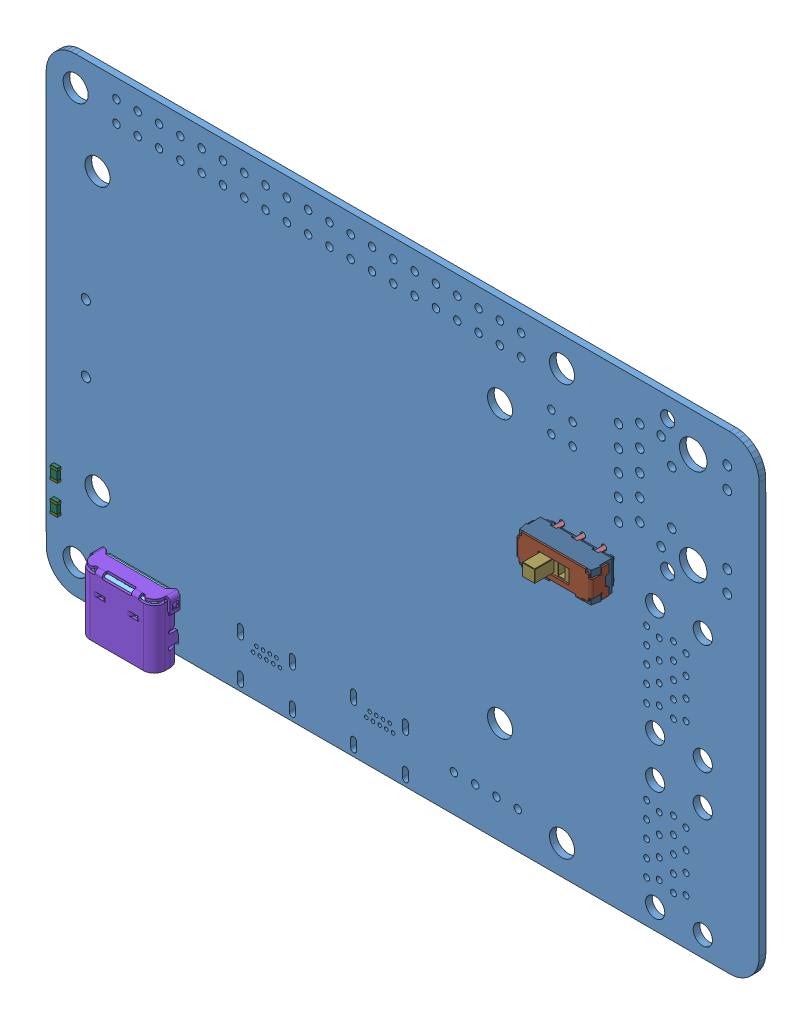
SolidWorks assembly CM4-to-Pi4-Adapter, configuration Default. Lengths in mm.
Overall size (85.02 56.9 9.11).
557 component instances, 55 part files, 0 mates.
Components (placement in the parent):
- CM4-to-Pi4-Adapter-3D.step-1: CM4-to-Pi4-Adapter-3D.step [Default] at origin size (85.02 56.9 9.11)
  - C56.step-1: C56.step [Default] at origin size (1.65 0.7 0.46)
    - 1028708016.step-1: 1028708016.step [Default] at (21.6693 15.4568 -1.2584) size (0.28 0.7 0.46)
      - Extruded.step-1: Extruded.step [Default] at origin size (0.28 0.7 0.46)
    - 1028708016.step-2: 1028708016.step [Default] at (20.2978 15.4568 -1.2584) size (0.28 0.7 0.46)
      - Extruded.step-1: Extruded.step [Default] at origin size (0.28 0.7 0.46)
    - 1028712752.step-1: 1028712752.step [Default] at (20.9835 15.4568 -1.2484) size (1.5 0.6 0.42)
      - Extruded-0.step-1: Extruded-0.step [Default] at origin size (1.5 0.6 0.42)
  - RJ1.step-1: RJ1.step [Default] at origin (suppressed, hidden)
  - C43.step-1: C43.step [Default] at origin size (1.65 0.7 0.46)
    - 1028708016.step-1: 1028708016.step [Default] at (79.781 44.229 -1.2584) size (0.28 0.7 0.46)
      - Extruded.step-1: Extruded.step [Default] at origin size (0.28 0.7 0.46)
    - 1028708016.step-2: 1028708016.step [Default] at (81.1525 44.229 -1.2584) size (0.28 0.7 0.46)
      - Extruded.step-1: Extruded.step [Default] at origin size (0.28 0.7 0.46)
    - 1028712752.step-1: 1028712752.step [Default] at (80.4667 44.229 -1.2484) size (1.5 0.6 0.42)
      - Extruded-0.step-1: Extruded-0.step [Default] at origin size (1.5 0.6 0.42)
  - U5.step-1: U5.step [Default] at origin size (7.8 5.3 2.16)
    - 1028708272.step-1: 1028708272.step [Default] at (47.5222 47.1882 -1.0524) size (1.3 0.41 0.25)
      - Extruded-6.step-1: Extruded-6.step [Default] at origin size (1.3 0.41 0.25)
    - 1028708272.step-2: 1028708272.step [Default] at (47.5222 45.9182 -1.0524) size (1.3 0.41 0.25)
      - Extruded-6.step-1: Extruded-6.step [Default] at origin size (1.3 0.41 0.25)
    - 1028708272.step-3: 1028708272.step [Default] at (47.5222 44.6482 -1.0524) size (1.3 0.41 0.25)
      - Extruded-6.step-1: Extruded-6.step [Default] at origin size (1.3 0.41 0.25)
    - 1028708272.step-4: 1028708272.step [Default] at (47.5222 43.3782 -1.0524) size (1.3 0.41 0.25)
      - Extruded-6.step-1: Extruded-6.step [Default] at origin size (1.3 0.41 0.25)
    - 1028708272.step-5: 1028708272.step [Default] at (41.0222 47.1982 -1.0524) size (1.3 0.41 0.25)
      - Extruded-6.step-1: Extruded-6.step [Default] at origin size (1.3 0.41 0.25)
    - 1028708272.step-6: 1028708272.step [Default] at (41.0222 45.9282 -1.0524) size (1.3 0.41 0.25)
      - Extruded-6.step-1: Extruded-6.step [Default] at origin size (1.3 0.41 0.25)
    - 1028708272.step-7: 1028708272.step [Default] at (41.0222 44.6582 -1.0524) size (1.3 0.41 0.25)
      - Extruded-6.step-1: Extruded-6.step [Default] at origin size (1.3 0.41 0.25)
    - 1028708272.step-8: 1028708272.step [Default] at (41.0222 43.3882 -1.0524) size (1.3 0.41 0.25)
      - Extruded-6.step-1: Extruded-6.step [Default] at origin size (1.3 0.41 0.25)
    - 1028710064.step-1: 1028710064.step [Default] at (44.2722 45.2882 -2.9584) size (5.4 5.3 2.01)
      - Extruded-7.step-1: Extruded-7.step [Default] at origin size (5.4 5.3 2.01)
  - Type_C1.step-1: Type_C1.step [Default] at origin size (9.58 7.71 4.16)
    - 698b116-264-211.step-1: 698b116-264-211.step [Default] at (-4.8722 -5.2197 -12) x (1 0 0) z (0 -1 0) size (9.58 4.16 7.71)
      - SOLID.step-1: SOLID.step [Default] at origin size (8.34 3.56 7.05)
      - SOLID-8.step-1: SOLID-8.step [Default] at origin size (0.26 1.45 0.87)
      - SOLID-9.step-1: SOLID-9.step [Default] at origin size (0.26 1.45 0.87)
      - SOLID-10.step-1: SOLID-10.step [Default] at origin size (0.25 1.45 0.87)
      - SOLID-11.step-1: SOLID-11.step [Default] at origin size (0.25 1.45 0.87)
      - SOLID-12.step-1: SOLID-12.step [Default] at origin size (0.25 2.03 6.58)
      - SOLID-13.step-1: SOLID-13.step [Default] at origin size (0.25 2.03 6.58)
      - SOLID-14.step-1: SOLID-14.step [Default] at origin size (0.25 1.57 6.58)
      - SOLID-15.step-1: SOLID-15.step [Default] at origin size (0.25 1.57 6.58)
      - SOLID-16.step-1: SOLID-16.step [Default] at origin size (0.25 0.24 5.71)
      - SOLID-17.step-1: SOLID-17.step [Default] at origin size (0.25 0.24 5.71)
      - SOLID-18.step-1: SOLID-18.step [Default] at origin size (0.85 1.57 7.13)
      - SOLID-19.step-1: SOLID-19.step [Default] at origin size (0.35 2.03 6.78)
      - SOLID-20.step-1: SOLID-20.step [Default] at origin size (0.35 0.24 5.91)
      - SOLID-21.step-1: SOLID-21.step [Default] at origin size (0.35 2.03 6.78)
      - SOLID-22.step-1: SOLID-22.step [Default] at origin size (0.35 0.24 5.91)
      - SOLID-23.step-1: SOLID-23.step [Default] at origin size (0.85 1.57 7.13)
      - SOLID-24.step-1: SOLID-24.step [Default] at origin size (0.25 0.24 4.21)
      - SOLID-25.step-1: SOLID-25.step [Default] at origin size (0.25 0.24 4.21)
      - SOLID-26.step-1: SOLID-26.step [Default] at origin size (1.11 2.03 7.13)
      - SOLID-27.step-1: SOLID-27.step [Default] at origin size (1.12 2.03 7.13)
      - SOLID-28.step-1: SOLID-28.step [Default] at origin size (9.58 4.16 7.53)
  - PWR4.step-1: PWR4.step [Default] at origin size (1.65 0.7 0.46)
    - 1028708016.step-1: 1028708016.step [Default] at (60.1471 9.525 -1.2584) size (0.28 0.7 0.46)
      - Extruded.step-1: Extruded.step [Default] at origin size (0.28 0.7 0.46)
    - 1028708016.step-2: 1028708016.step [Default] at (61.5187 9.525 -1.2584) size (0.28 0.7 0.46)
      - Extruded.step-1: Extruded.step [Default] at origin size (0.28 0.7 0.46)
    - 1028712752.step-1: 1028712752.step [Default] at (60.8329 9.525 -1.2484) size (1.5 0.6 0.42)
      - Extruded-0.step-1: Extruded-0.step [Default] at origin size (1.5 0.6 0.42)
  - J2.step-1: J2.step [Default] at origin (suppressed, hidden)
  - J1.step-1: J1.step [Default] at origin (suppressed, hidden)
  - I1.step-1: I1.step [Default] at origin size (1.2 2.3 1.1)
    - User_Library-1N4148WS.step-1: User_Library-1N4148WS.step [Default] at (45.6439 39.5224 -1.05) x (0 -1 0) z (0 0 1) size (2.3 1.2 1.1)
  - U6.step-1: U6.step [Default] at origin size (8.1 8.1 0.83)
    - 1028701360.step-1: 1028701360.step [Default] at (46.9011 27.4447 -1.6484) size (8.1 8.1 0.83)
      - Extruded-53.step-1: Extruded-53.step [Default] at origin size (8.1 8.1 0.83)
  - PWR3.step-1: PWR3.step [Default] at origin size (1.65 0.85 0.46)
    - 1032565968.step-1: 1032565968.step [Default] at (60.7531 10.7826 -1.2484) size (1.5 0.8 0.42)
      - Extruded-54.step-1: Extruded-54.step [Default] at origin size (1.5 0.8 0.42)
    - 1032565712.step-1: 1032565712.step [Default] at (60.0673 10.7826 -1.2584) size (0.28 0.85 0.46)
      - Extruded-55.step-1: Extruded-55.step [Default] at origin size (0.28 0.85 0.46)
    - 1032565712.step-2: 1032565712.step [Default] at (61.4388 10.7826 -1.2584) size (0.28 0.85 0.46)
      - Extruded-55.step-1: Extruded-55.step [Default] at origin size (0.28 0.85 0.46)
  - PWR2.step-1: PWR2.step [Default] at origin size (0.7 1.65 0.46)
    - 1028703920.step-1: 1028703920.step [Default] at (53.2384 19.7867 -1.2584) size (0.7 0.28 0.46)
      - Extruded-56.step-1: Extruded-56.step [Default] at origin size (0.7 0.28 0.46)
    - 1028703920.step-2: 1028703920.step [Default] at (53.2384 18.4151 -1.2584) size (0.7 0.28 0.46)
      - Extruded-56.step-1: Extruded-56.step [Default] at origin size (0.7 0.28 0.46)
    - 1032570704.step-1: 1032570704.step [Default] at (53.2384 19.1009 -1.2484) size (0.6 1.5 0.42)
      - Extruded-57.step-1: Extruded-57.step [Default] at origin size (0.6 1.5 0.42)
  - PWR1.step-1: PWR1.step [Default] at origin size (0.85 1.65 0.46)
    - 1032565072.step-1: 1032565072.step [Default] at (54.5845 19.0753 -1.2484) size (0.8 1.5 0.42)
      - Extruded-58.step-1: Extruded-58.step [Default] at origin size (0.8 1.5 0.42)
    - 1032568144.step-1: 1032568144.step [Default] at (54.5845 19.7611 -1.2584) size (0.85 0.28 0.46)
      - Extruded-59.step-1: Extruded-59.step [Default] at origin size (0.85 0.28 0.46)
    - 1032568144.step-2: 1032568144.step [Default] at (54.5845 18.3896 -1.2584) size (0.85 0.28 0.46)
      - Extruded-59.step-1: Extruded-59.step [Default] at origin size (0.85 0.28 0.46)
  - C55.step-1: C55.step [Default] at origin size (0.85 1.65 0.46)
    - 1032568144.step-1: 1032568144.step [Default] at (8.4022 6.793 -1.2584) size (0.85 0.28 0.46)
      - Extruded-59.step-1: Extruded-59.step [Default] at origin size (0.85 0.28 0.46)
    - 1032568144.step-2: 1032568144.step [Default] at (8.4022 8.1646 -1.2584) size (0.85 0.28 0.46)
      - Extruded-59.step-1: Extruded-59.step [Default] at origin size (0.85 0.28 0.46)
    - 1032565072.step-1: 1032565072.step [Default] at (8.4022 7.4787 -1.2484) size (0.8 1.5 0.42)
      - Extruded-58.step-1: Extruded-58.step [Default] at origin size (0.8 1.5 0.42)
  - C54.step-1: C54.step [Default] at origin size (0.85 1.65 0.46)
    - 1032568144.step-1: 1032568144.step [Default] at (39.5479 19.754 -1.2584) size (0.85 0.28 0.46)
      - Extruded-59.step-1: Extruded-59.step [Default] at origin size (0.85 0.28 0.46)
    - 1032568144.step-2: 1032568144.step [Default] at (39.5479 18.3825 -1.2584) size (0.85 0.28 0.46)
      - Extruded-59.step-1: Extruded-59.step [Default] at origin size (0.85 0.28 0.46)
    - 1032565072.step-1: 1032565072.step [Default] at (39.5479 19.0683 -1.2484) size (0.8 1.5 0.42)
      - Extruded-58.step-1: Extruded-58.step [Default] at origin size (0.8 1.5 0.42)
  - C53.step-1: C53.step [Default] at origin size (1.65 0.85 0.46)
    - 1032565712.step-1: 1032565712.step [Default] at (47.5691 18.4938 -1.2584) size (0.28 0.85 0.46)
      - Extruded-55.step-1: Extruded-55.step [Default] at origin size (0.28 0.85 0.46)
    - 1032565712.step-2: 1032565712.step [Default] at (46.1976 18.4938 -1.2584) size (0.28 0.85 0.46)
      - Extruded-55.step-1: Extruded-55.step [Default] at origin size (0.28 0.85 0.46)
    - 1032565968.step-1: 1032565968.step [Default] at (46.8834 18.4938 -1.2484) size (1.5 0.8 0.42)
      - Extruded-54.step-1: Extruded-54.step [Default] at origin size (1.5 0.8 0.42)
  - C52.step-1: C52.step [Default] at origin size (1.65 0.7 0.46)
    - 1028708016.step-1: 1028708016.step [Default] at (53.2841 32.3371 -1.2584) size (0.28 0.7 0.46)
      - Extruded.step-1: Extruded.step [Default] at origin size (0.28 0.7 0.46)
    - 1028708016.step-2: 1028708016.step [Default] at (54.6556 32.3371 -1.2584) size (0.28 0.7 0.46)
      - Extruded.step-1: Extruded.step [Default] at origin size (0.28 0.7 0.46)
    - 1028712752.step-1: 1028712752.step [Default] at (53.9699 32.3371 -1.2484) size (1.5 0.6 0.42)
      - Extruded-0.step-1: Extruded-0.step [Default] at origin size (1.5 0.6 0.42)
  - C51.step-1: C51.step [Default] at origin size (0.7 1.65 0.46)
    - 1028703920.step-1: 1028703920.step [Default] at (44.5186 19.746 -1.2584) size (0.7 0.28 0.46)
      - Extruded-56.step-1: Extruded-56.step [Default] at origin size (0.7 0.28 0.46)
    - 1028703920.step-2: 1028703920.step [Default] at (44.5186 18.3745 -1.2584) size (0.7 0.28 0.46)
      - Extruded-56.step-1: Extruded-56.step [Default] at origin size (0.7 0.28 0.46)
    - 1032570704.step-1: 1032570704.step [Default] at (44.5186 19.0602 -1.2484) size (0.6 1.5 0.42)
      - Extruded-57.step-1: Extruded-57.step [Default] at origin size (0.6 1.5 0.42)
  - C50.step-1: C50.step [Default] at origin size (0.7 1.65 0.46)
    - 1028703920.step-1: 1028703920.step [Default] at (42.1519 19.746 -1.2584) size (0.7 0.28 0.46)
      - Extruded-56.step-1: Extruded-56.step [Default] at origin size (0.7 0.28 0.46)
    - 1028703920.step-2: 1028703920.step [Default] at (42.1519 18.3745 -1.2584) size (0.7 0.28 0.46)
      - Extruded-56.step-1: Extruded-56.step [Default] at origin size (0.7 0.28 0.46)
    - 1032570704.step-1: 1032570704.step [Default] at (42.1519 19.0602 -1.2484) size (0.6 1.5 0.42)
      - Extruded-57.step-1: Extruded-57.step [Default] at origin size (0.6 1.5 0.42)
  - C49.step-1: C49.step [Default] at origin size (0.7 1.65 0.46)
    - 1028703920.step-1: 1028703920.step [Default] at (43.3352 19.746 -1.2584) size (0.7 0.28 0.46)
      - Extruded-56.step-1: Extruded-56.step [Default] at origin size (0.7 0.28 0.46)
    - 1028703920.step-2: 1028703920.step [Default] at (43.3352 18.3745 -1.2584) size (0.7 0.28 0.46)
      - Extruded-56.step-1: Extruded-56.step [Default] at origin size (0.7 0.28 0.46)
    - 1032570704.step-1: 1032570704.step [Default] at (43.3352 19.0602 -1.2484) size (0.6 1.5 0.42)
      - Extruded-57.step-1: Extruded-57.step [Default] at origin size (0.6 1.5 0.42)
  - C48.step-1: C48.step [Default] at origin size (0.7 1.65 0.46)
    - 1028703920.step-1: 1028703920.step [Default] at (49.2404 19.746 -1.2584) size (0.7 0.28 0.46)
      - Extruded-56.step-1: Extruded-56.step [Default] at origin size (0.7 0.28 0.46)
    - 1028703920.step-2: 1028703920.step [Default] at (49.2404 18.3745 -1.2584) size (0.7 0.28 0.46)
      - Extruded-56.step-1: Extruded-56.step [Default] at origin size (0.7 0.28 0.46)
    - 1032570704.step-1: 1032570704.step [Default] at (49.2404 19.0602 -1.2484) size (0.6 1.5 0.42)
      - Extruded-57.step-1: Extruded-57.step [Default] at origin size (0.6 1.5 0.42)
  - C47.step-1: C47.step [Default] at origin size (0.7 1.65 0.46)
    - 1028703920.step-1: 1028703920.step [Default] at (43.3429 34.5262 -1.2584) size (0.7 0.28 0.46)
      - Extruded-56.step-1: Extruded-56.step [Default] at origin size (0.7 0.28 0.46)
    - 1028703920.step-2: 1028703920.step [Default] at (43.3429 35.8977 -1.2584) size (0.7 0.28 0.46)
      - Extruded-56.step-1: Extruded-56.step [Default] at origin size (0.7 0.28 0.46)
    - 1032570704.step-1: 1032570704.step [Default] at (43.3429 35.212 -1.2484) size (0.6 1.5 0.42)
      - Extruded-57.step-1: Extruded-57.step [Default] at origin size (0.6 1.5 0.42)
  - C46.step-1: C46.step [Default] at origin size (1.65 0.7 0.46)
    - 1028708016.step-1: 1028708016.step [Default] at (47.5692 19.812 -1.2584) size (0.28 0.7 0.46)
      - Extruded.step-1: Extruded.step [Default] at origin size (0.28 0.7 0.46)
    - 1028708016.step-2: 1028708016.step [Default] at (46.1976 19.812 -1.2584) size (0.28 0.7 0.46)
      - Extruded.step-1: Extruded.step [Default] at origin size (0.28 0.7 0.46)
    - 1028712752.step-1: 1028712752.step [Default] at (46.8834 19.812 -1.2484) size (1.5 0.6 0.42)
      - Extruded-0.step-1: Extruded-0.step [Default] at origin size (1.5 0.6 0.42)
  - C45.step-1: C45.step [Default] at origin size (1.65 0.7 0.46)
    - 1028708016.step-1: 1028708016.step [Default] at (38.7807 25.7962 -1.2584) size (0.28 0.7 0.46)
      - Extruded.step-1: Extruded.step [Default] at origin size (0.28 0.7 0.46)
    - 1028708016.step-2: 1028708016.step [Default] at (40.1522 25.7962 -1.2584) size (0.28 0.7 0.46)
      - Extruded.step-1: Extruded.step [Default] at origin size (0.28 0.7 0.46)
    - 1028712752.step-1: 1028712752.step [Default] at (39.4664 25.7962 -1.2484) size (1.5 0.6 0.42)
      - Extruded-0.step-1: Extruded-0.step [Default] at origin size (1.5 0.6 0.42)
  - C44.step-1: C44.step [Default] at origin size (1.65 0.7 0.46)
    - 1028708016.step-1: 1028708016.step [Default] at (38.7858 26.8605 -1.2584) size (0.28 0.7 0.46)
      - Extruded.step-1: Extruded.step [Default] at origin size (0.28 0.7 0.46)
    - 1028708016.step-2: 1028708016.step [Default] at (40.1573 26.8605 -1.2584) size (0.28 0.7 0.46)
      - Extruded.step-1: Extruded.step [Default] at origin size (0.28 0.7 0.46)
    - 1028712752.step-1: 1028712752.step [Default] at (39.4715 26.8605 -1.2484) size (1.5 0.6 0.42)
      - Extruded-0.step-1: Extruded-0.step [Default] at origin size (1.5 0.6 0.42)
  - C42.step-1: C42.step [Default] at origin size (1.65 0.7 0.46)
    - 1028708016.step-1: 1028708016.step [Default] at (38.7263 28.1998 -1.2584) size (0.28 0.7 0.46)
      - Extruded.step-1: Extruded.step [Default] at origin size (0.28 0.7 0.46)
    - 1028708016.step-2: 1028708016.step [Default] at (40.0979 28.1998 -1.2584) size (0.28 0.7 0.46)
      - Extruded.step-1: Extruded.step [Default] at origin size (0.28 0.7 0.46)
    - 1028712752.step-1: 1028712752.step [Default] at (39.4121 28.1998 -1.2484) size (1.5 0.6 0.42)
      - Extruded-0.step-1: Extruded-0.step [Default] at origin size (1.5 0.6 0.42)
  - C41.step-1: C41.step [Default] at origin size (1.65 0.7 0.46)
    - 1028708016.step-1: 1028708016.step [Default] at (38.7349 29.243 -1.2584) size (0.28 0.7 0.46)
      - Extruded.step-1: Extruded.step [Default] at origin size (0.28 0.7 0.46)
    - 1028708016.step-2: 1028708016.step [Default] at (40.1065 29.243 -1.2584) size (0.28 0.7 0.46)
      - Extruded.step-1: Extruded.step [Default] at origin size (0.28 0.7 0.46)
    - 1028712752.step-1: 1028712752.step [Default] at (39.4207 29.243 -1.2484) size (1.5 0.6 0.42)
      - Extruded-0.step-1: Extruded-0.step [Default] at origin size (1.5 0.6 0.42)
  - C40.step-1: C40.step [Default] at origin size (0.85 1.65 0.46)
    - 1032565072.step-1: 1032565072.step [Default] at (51.1555 35.2043 -1.2484) size (0.8 1.5 0.42)
      - Extruded-58.step-1: Extruded-58.step [Default] at origin size (0.8 1.5 0.42)
    - 1032568144.step-1: 1032568144.step [Default] at (51.1555 35.8901 -1.2584) size (0.85 0.28 0.46)
      - Extruded-59.step-1: Extruded-59.step [Default] at origin size (0.85 0.28 0.46)
    - 1032568144.step-2: 1032568144.step [Default] at (51.1555 34.5186 -1.2584) size (0.85 0.28 0.46)
      - Extruded-59.step-1: Extruded-59.step [Default] at origin size (0.85 0.28 0.46)
  - C39.step-1: C39.step [Default] at origin size (1.65 0.7 0.46)
    - 1028708016.step-1: 1028708016.step [Default] at (40.1626 31.1912 -1.2584) size (0.28 0.7 0.46)
      - Extruded.step-1: Extruded.step [Default] at origin size (0.28 0.7 0.46)
    - 1028708016.step-2: 1028708016.step [Default] at (38.791 31.1912 -1.2584) size (0.28 0.7 0.46)
      - Extruded.step-1: Extruded.step [Default] at origin size (0.28 0.7 0.46)
    - 1028712752.step-1: 1028712752.step [Default] at (39.4767 31.1912 -1.2484) size (1.5 0.6 0.42)
      - Extruded-0.step-1: Extruded-0.step [Default] at origin size (1.5 0.6 0.42)
  - C38.step-1: C38.step [Default] at origin size (1.65 0.7 0.46)
    - 1028708016.step-1: 1028708016.step [Default] at (40.2336 23.3096 -1.2584) size (0.28 0.7 0.46)
      - Extruded.step-1: Extruded.step [Default] at origin size (0.28 0.7 0.46)
    - 1028708016.step-2: 1028708016.step [Default] at (38.8621 23.3096 -1.2584) size (0.28 0.7 0.46)
      - Extruded.step-1: Extruded.step [Default] at origin size (0.28 0.7 0.46)
    - 1028712752.step-1: 1028712752.step [Default] at (39.5478 23.3096 -1.2484) size (1.5 0.6 0.42)
      - Extruded-0.step-1: Extruded-0.step [Default] at origin size (1.5 0.6 0.42)
  - C37.step-1: C37.step [Default] at origin size (0.7 1.65 0.46)
    - 1028703920.step-1: 1028703920.step [Default] at (50.5973 19.746 -1.2584) size (0.7 0.28 0.46)
      - Extruded-56.step-1: Extruded-56.step [Default] at origin size (0.7 0.28 0.46)
    - 1028703920.step-2: 1028703920.step [Default] at (50.5973 18.3745 -1.2584) size (0.7 0.28 0.46)
      - Extruded-56.step-1: Extruded-56.step [Default] at origin size (0.7 0.28 0.46)
    - 1032570704.step-1: 1032570704.step [Default] at (50.5973 19.0602 -1.2484) size (0.6 1.5 0.42)
      - Extruded-57.step-1: Extruded-57.step [Default] at origin size (0.6 1.5 0.42)
  - C36.step-1: C36.step [Default] at origin size (0.7 1.65 0.46)
    - 1028703920.step-1: 1028703920.step [Default] at (51.9542 19.746 -1.2584) size (0.7 0.28 0.46)
      - Extruded-56.step-1: Extruded-56.step [Default] at origin size (0.7 0.28 0.46)
    - 1028703920.step-2: 1028703920.step [Default] at (51.9542 18.3745 -1.2584) size (0.7 0.28 0.46)
      - Extruded-56.step-1: Extruded-56.step [Default] at origin size (0.7 0.28 0.46)
    - 1032570704.step-1: 1032570704.step [Default] at (51.9542 19.0602 -1.2484) size (0.6 1.5 0.42)
      - Extruded-57.step-1: Extruded-57.step [Default] at origin size (0.6 1.5 0.42)
  - C35.step-1: C35.step [Default] at origin size (1.65 0.7 0.46)
    - 1028708016.step-1: 1028708016.step [Default] at (53.2892 33.4826 -1.2584) size (0.28 0.7 0.46)
      - Extruded.step-1: Extruded.step [Default] at origin size (0.28 0.7 0.46)
    - 1028708016.step-2: 1028708016.step [Default] at (54.6608 33.4826 -1.2584) size (0.28 0.7 0.46)
      - Extruded.step-1: Extruded.step [Default] at origin size (0.28 0.7 0.46)
    - 1028712752.step-1: 1028712752.step [Default] at (53.975 33.4826 -1.2484) size (1.5 0.6 0.42)
      - Extruded-0.step-1: Extruded-0.step [Default] at origin size (1.5 0.6 0.42)
  - C34.step-1: C34.step [Default] at origin size (1.65 0.7 0.46)
    - 1028708016.step-1: 1028708016.step [Default] at (53.2841 22.2834 -1.2584) size (0.28 0.7 0.46)
      - Extruded.step-1: Extruded.step [Default] at origin size (0.28 0.7 0.46)
    - 1028708016.step-2: 1028708016.step [Default] at (54.6556 22.2834 -1.2584) size (0.28 0.7 0.46)
      - Extruded.step-1: Extruded.step [Default] at origin size (0.28 0.7 0.46)
    - 1028712752.step-1: 1028712752.step [Default] at (53.9699 22.2834 -1.2484) size (1.5 0.6 0.42)
      - Extruded-0.step-1: Extruded-0.step [Default] at origin size (1.5 0.6 0.42)
  - C33.step-1: C33.step [Default] at origin size (1.65 0.7 0.46)
    - 1028708016.step-1: 1028708016.step [Default] at (53.2581 21.1786 -1.2584) size (0.28 0.7 0.46)
      - Extruded.step-1: Extruded.step [Default] at origin size (0.28 0.7 0.46)
    - 1028708016.step-2: 1028708016.step [Default] at (54.6296 21.1786 -1.2584) size (0.28 0.7 0.46)
      - Extruded.step-1: Extruded.step [Default] at origin size (0.28 0.7 0.46)
    - 1028712752.step-1: 1028712752.step [Default] at (53.9439 21.1786 -1.2484) size (1.5 0.6 0.42)
      - Extruded-0.step-1: Extruded-0.step [Default] at origin size (1.5 0.6 0.42)
  - AMS-1.step-1: AMS-1.step [Default] at origin size (6.73 3.43 1.02)
    - 1032565584.step-1: 1032565584.step [Default] at (60.7466 16.1548 -2.0684) size (6.73 3.43 1.02)
      - Extruded-60.step-1: Extruded-60.step [Default] at origin size (6.73 3.43 1.02)
  - C9.step-1: C9.step [Default] at origin size (0.7 1.65 0.46)
    - 1028703920.step-1: 1028703920.step [Default] at (38.585 45.8952 -1.2584) size (0.7 0.28 0.46)
      - Extruded-56.step-1: Extruded-56.step [Default] at origin size (0.7 0.28 0.46)
    - 1028703920.step-2: 1028703920.step [Default] at (38.585 47.2668 -1.2584) size (0.7 0.28 0.46)
      - Extruded-56.step-1: Extruded-56.step [Default] at origin size (0.7 0.28 0.46)
    - 1032570704.step-1: 1032570704.step [Default] at (38.585 46.581 -1.2484) size (0.6 1.5 0.42)
      - Extruded-57.step-1: Extruded-57.step [Default] at origin size (0.6 1.5 0.42)
  - C23.step-1: C23.step [Default] at origin size (1.6 0.8 0.6)
    - CAPC1608(0603).step-1: CAPC1608(0603).step [Default] at (20.9711 17.8537 -0.7984) x (-1 0 0) z (0 0 -1) size (1.6 0.8 0.6)
  - P3.step-1: P3.step [Default] at origin (suppressed, hidden)
  - C32.step-1: C32.step [Default] at origin size (0.7 1.65 0.46)
    - 1028703920.step-1: 1028703920.step [Default] at (47.0662 38.9381 -1.2584) size (0.7 0.28 0.46)
      - Extruded-56.step-1: Extruded-56.step [Default] at origin size (0.7 0.28 0.46)
    - 1028703920.step-2: 1028703920.step [Default] at (47.0662 40.3097 -1.2584) size (0.7 0.28 0.46)
      - Extruded-56.step-1: Extruded-56.step [Default] at origin size (0.7 0.28 0.46)
    - 1032570704.step-1: 1032570704.step [Default] at (47.0662 39.6239 -1.2484) size (0.6 1.5 0.42)
      - Extruded-57.step-1: Extruded-57.step [Default] at origin size (0.6 1.5 0.42)
  - C31.step-1: C31.step [Default] at origin size (0.7 1.65 0.46)
    - 1028703920.step-1: 1028703920.step [Default] at (49.9161 34.5262 -1.2584) size (0.7 0.28 0.46)
      - Extruded-56.step-1: Extruded-56.step [Default] at origin size (0.7 0.28 0.46)
    - 1028703920.step-2: 1028703920.step [Default] at (49.9161 35.8977 -1.2584) size (0.7 0.28 0.46)
      - Extruded-56.step-1: Extruded-56.step [Default] at origin size (0.7 0.28 0.46)
    - 1032570704.step-1: 1032570704.step [Default] at (49.9161 35.212 -1.2484) size (0.6 1.5 0.42)
      - Extruded-57.step-1: Extruded-57.step [Default] at origin size (0.6 1.5 0.42)
  - C30.step-1: C30.step [Default] at origin size (0.7 1.65 0.46)
    - 1028703920.step-1: 1028703920.step [Default] at (44.45 35.8979 -1.2584) size (0.7 0.28 0.46)
      - Extruded-56.step-1: Extruded-56.step [Default] at origin size (0.7 0.28 0.46)
    - 1028703920.step-2: 1028703920.step [Default] at (44.45 34.5263 -1.2584) size (0.7 0.28 0.46)
      - Extruded-56.step-1: Extruded-56.step [Default] at origin size (0.7 0.28 0.46)
    - 1032570704.step-1: 1032570704.step [Default] at (44.45 35.2121 -1.2484) size (0.6 1.5 0.42)
      - Extruded-57.step-1: Extruded-57.step [Default] at origin size (0.6 1.5 0.42)
  - C29.step-1: C29.step [Default] at origin size (1.65 0.7 0.46)
    - 1028708016.step-1: 1028708016.step [Default] at (67.3967 2.4784 -1.2584) size (0.28 0.7 0.46)
      - Extruded.step-1: Extruded.step [Default] at origin size (0.28 0.7 0.46)
    - 1028708016.step-2: 1028708016.step [Default] at (68.7683 2.4784 -1.2584) size (0.28 0.7 0.46)
      - Extruded.step-1: Extruded.step [Default] at origin size (0.28 0.7 0.46)
    - 1028712752.step-1: 1028712752.step [Default] at (68.0825 2.4784 -1.2484) size (1.5 0.6 0.42)
      - Extruded-0.step-1: Extruded-0.step [Default] at origin size (1.5 0.6 0.42)
  - C28.step-1: C28.step [Default] at origin size (1.65 0.7 0.46)
    - 1028708016.step-1: 1028708016.step [Default] at (67.3734 20.2642 -1.2584) size (0.28 0.7 0.46)
      - Extruded.step-1: Extruded.step [Default] at origin size (0.28 0.7 0.46)
    - 1028708016.step-2: 1028708016.step [Default] at (68.745 20.2642 -1.2584) size (0.28 0.7 0.46)
      - Extruded.step-1: Extruded.step [Default] at origin size (0.28 0.7 0.46)
    - 1028712752.step-1: 1028712752.step [Default] at (68.0592 20.2642 -1.2484) size (1.5 0.6 0.42)
      - Extruded-0.step-1: Extruded-0.step [Default] at origin size (1.5 0.6 0.42)
  - C27.step-1: C27.step [Default] at origin size (1.65 0.7 0.46)
    - 1028708016.step-1: 1028708016.step [Default] at (67.3734 3.5883 -1.2584) size (0.28 0.7 0.46)
      - Extruded.step-1: Extruded.step [Default] at origin size (0.28 0.7 0.46)
    - 1028708016.step-2: 1028708016.step [Default] at (68.745 3.5883 -1.2584) size (0.28 0.7 0.46)
      - Extruded.step-1: Extruded.step [Default] at origin size (0.28 0.7 0.46)
    - 1028712752.step-1: 1028712752.step [Default] at (68.0592 3.5883 -1.2484) size (1.5 0.6 0.42)
      - Extruded-0.step-1: Extruded-0.step [Default] at origin size (1.5 0.6 0.42)
  - U3.step-1: U3.step [Default] at origin size (1.81 1.7 0.55)
    - 1028711728.step-1: 1028711728.step [Default] at (18.5512 13.9889 -0.9584) size (0.4 0.23 0.16)
      - Extruded-61.step-1: Extruded-61.step [Default] at origin size (0.4 0.23 0.16)
    - 1028711728.step-2: 1028711728.step [Default] at (18.5512 14.4889 -0.9584) size (0.4 0.23 0.16)
      - Extruded-61.step-1: Extruded-61.step [Default] at origin size (0.4 0.23 0.16)
    - 1028711728.step-3: 1028711728.step [Default] at (18.5512 14.9889 -0.9584) size (0.4 0.23 0.16)
      - Extruded-61.step-1: Extruded-61.step [Default] at origin size (0.4 0.23 0.16)
    - 1028711728.step-4: 1028711728.step [Default] at (17.1491 14.9889 -0.9584) size (0.4 0.23 0.16)
      - Extruded-61.step-1: Extruded-61.step [Default] at origin size (0.4 0.23 0.16)
    - 1028711728.step-5: 1028711728.step [Default] at (17.1491 14.4889 -0.9584) size (0.4 0.23 0.16)
      - Extruded-61.step-1: Extruded-61.step [Default] at origin size (0.4 0.23 0.16)
    - 1028711728.step-6: 1028711728.step [Default] at (17.1491 13.9889 -0.9584) size (0.4 0.23 0.16)
      - Extruded-61.step-1: Extruded-61.step [Default] at origin size (0.4 0.23 0.16)
    - 1032567248.step-1: 1032567248.step [Default] at (17.8513 14.489 -1.3484) size (1.3 1.7 0.5)
      - Extruded-62.step-1: Extruded-62.step [Default] at origin size (1.3 1.7 0.5)
  - L3.step-1: L3.step [Default] at origin size (0.85 1.52 0.46)
    - 1032568144.step-1: 1032568144.step [Default] at (1.35 7.6497 0.001) size (0.85 0.28 0.46)
      - Extruded-59.step-1: Extruded-59.step [Default] at origin size (0.85 0.28 0.46)
    - 1032568144.step-2: 1032568144.step [Default] at (1.35 8.8739 0.001) size (0.85 0.28 0.46)
      - Extruded-59.step-1: Extruded-59.step [Default] at origin size (0.85 0.28 0.46)
    - 1032565072.step-1: 1032565072.step [Default] at (1.35 8.2872 0.025) size (0.8 1.5 0.42)
      - Extruded-58.step-1: Extruded-58.step [Default] at origin size (0.8 1.5 0.42)
  - C26.step-1: C26.step [Default] at origin size (1.65 0.7 0.46)
    - 1028708016.step-1: 1028708016.step [Default] at (17.0687 8.095 -1.2584) size (0.28 0.7 0.46)
      - Extruded.step-1: Extruded.step [Default] at origin size (0.28 0.7 0.46)
    - 1028708016.step-2: 1028708016.step [Default] at (18.4403 8.095 -1.2584) size (0.28 0.7 0.46)
      - Extruded.step-1: Extruded.step [Default] at origin size (0.28 0.7 0.46)
    - 1028712752.step-1: 1028712752.step [Default] at (17.7545 8.095 -1.2484) size (1.5 0.6 0.42)
      - Extruded-0.step-1: Extruded-0.step [Default] at origin size (1.5 0.6 0.42)
  - C25.step-1: C25.step [Default] at origin size (1.65 0.7 0.46)
    - 1028708016.step-1: 1028708016.step [Default] at (17.0509 7.0688 -1.2584) size (0.28 0.7 0.46)
      - Extruded.step-1: Extruded.step [Default] at origin size (0.28 0.7 0.46)
    - 1028708016.step-2: 1028708016.step [Default] at (18.4225 7.0688 -1.2584) size (0.28 0.7 0.46)
      - Extruded.step-1: Extruded.step [Default] at origin size (0.28 0.7 0.46)
    - 1028712752.step-1: 1028712752.step [Default] at (17.7368 7.0688 -1.2484) size (1.5 0.6 0.42)
      - Extruded-0.step-1: Extruded-0.step [Default] at origin size (1.5 0.6 0.42)
  - C15.step-1: C15.step [Default] at origin size (1.65 0.7 0.46)
    - 1028708016.step-1: 1028708016.step [Default] at (6.7565 16.5354 -1.2584) size (0.28 0.7 0.46)
      - Extruded.step-1: Extruded.step [Default] at origin size (0.28 0.7 0.46)
    - 1028708016.step-2: 1028708016.step [Default] at (5.3849 16.5354 -1.2584) size (0.28 0.7 0.46)
      - Extruded.step-1: Extruded.step [Default] at origin size (0.28 0.7 0.46)
    - 1028712752.step-1: 1028712752.step [Default] at (6.0707 16.5354 -1.2484) size (1.5 0.6 0.42)
      - Extruded-0.step-1: Extruded-0.step [Default] at origin size (1.5 0.6 0.42)
  - C14.step-1: C14.step [Default] at origin size (1.65 0.85 0.46)
    - 1032565712.step-1: 1032565712.step [Default] at (6.7565 17.9069 -1.2584) size (0.28 0.85 0.46)
      - Extruded-55.step-1: Extruded-55.step [Default] at origin size (0.28 0.85 0.46)
    - 1032565712.step-2: 1032565712.step [Default] at (5.3849 17.9069 -1.2584) size (0.28 0.85 0.46)
      - Extruded-55.step-1: Extruded-55.step [Default] at origin size (0.28 0.85 0.46)
    - 1032565968.step-1: 1032565968.step [Default] at (6.0707 17.9069 -1.2484) size (1.5 0.8 0.42)
      - Extruded-54.step-1: Extruded-54.step [Default] at origin size (1.5 0.8 0.42)
  - C11.step-1: C11.step [Default] at origin size (0.85 1.65 0.46)
    - 1032568144.step-1: 1032568144.step [Default] at (17.356 12.4768 -1.2584) size (0.85 0.28 0.46)
      - Extruded-59.step-1: Extruded-59.step [Default] at origin size (0.85 0.28 0.46)
    - 1032568144.step-2: 1032568144.step [Default] at (17.356 11.1052 -1.2584) size (0.85 0.28 0.46)
      - Extruded-59.step-1: Extruded-59.step [Default] at origin size (0.85 0.28 0.46)
    - 1032565072.step-1: 1032565072.step [Default] at (17.356 11.791 -1.2484) size (0.8 1.5 0.42)
      - Extruded-58.step-1: Extruded-58.step [Default] at origin size (0.8 1.5 0.42)
  - C10.step-1: C10.step [Default] at origin size (0.7 1.65 0.46)
    - 1028703920.step-1: 1028703920.step [Default] at (17.356 17.968 -1.2584) size (0.7 0.28 0.46)
      - Extruded-56.step-1: Extruded-56.step [Default] at origin size (0.7 0.28 0.46)
    - 1028703920.step-2: 1028703920.step [Default] at (17.356 16.5965 -1.2584) size (0.7 0.28 0.46)
      - Extruded-56.step-1: Extruded-56.step [Default] at origin size (0.7 0.28 0.46)
    - 1032570704.step-1: 1032570704.step [Default] at (17.356 17.2822 -1.2484) size (0.6 1.5 0.42)
      - Extruded-57.step-1: Extruded-57.step [Default] at origin size (0.6 1.5 0.42)
  - C13.step-1: C13.step [Default] at origin size (1.65 0.7 0.46)
    - 1028708016.step-1: 1028708016.step [Default] at (20.2976 11.0917 -1.2584) size (0.28 0.7 0.46)
      - Extruded.step-1: Extruded.step [Default] at origin size (0.28 0.7 0.46)
    - 1028708016.step-2: 1028708016.step [Default] at (21.6692 11.0917 -1.2584) size (0.28 0.7 0.46)
      - Extruded.step-1: Extruded.step [Default] at origin size (0.28 0.7 0.46)
    - 1028712752.step-1: 1028712752.step [Default] at (20.9834 11.0917 -1.2484) size (1.5 0.6 0.42)
      - Extruded-0.step-1: Extruded-0.step [Default] at origin size (1.5 0.6 0.42)
  - Y1.step-1: Y1.step [Default] at origin size (3.95 3.1 1)
    - 1028712112.step-1: 1028712112.step [Default] at (47.1936 35.2552 -1.7984) size (3.95 3.1 1)
      - Extruded-63.step-1: Extruded-63.step [Default] at origin size (3.95 3.1 1)
  - C4.step-1: C4.step [Default] at origin size (0.7 1.65 0.46)
    - 1028703920.step-1: 1028703920.step [Default] at (47.1806 14.732 -1.2584) size (0.7 0.28 0.46)
      - Extruded-56.step-1: Extruded-56.step [Default] at origin size (0.7 0.28 0.46)
    - 1028703920.step-2: 1028703920.step [Default] at (47.1806 13.3604 -1.2584) size (0.7 0.28 0.46)
      - Extruded-56.step-1: Extruded-56.step [Default] at origin size (0.7 0.28 0.46)
    - 1032570704.step-1: 1032570704.step [Default] at (47.1806 14.0462 -1.2484) size (0.6 1.5 0.42)
      - Extruded-57.step-1: Extruded-57.step [Default] at origin size (0.6 1.5 0.42)
  - C3.step-1: C3.step [Default] at origin size (0.7 1.65 0.46)
    - 1028703920.step-1: 1028703920.step [Default] at (48.3412 13.3603 -1.2584) size (0.7 0.28 0.46)
      - Extruded-56.step-1: Extruded-56.step [Default] at origin size (0.7 0.28 0.46)
    - 1028703920.step-2: 1028703920.step [Default] at (48.3412 14.7318 -1.2584) size (0.7 0.28 0.46)
      - Extruded-56.step-1: Extruded-56.step [Default] at origin size (0.7 0.28 0.46)
    - 1032570704.step-1: 1032570704.step [Default] at (48.3412 14.0461 -1.2484) size (0.6 1.5 0.42)
      - Extruded-57.step-1: Extruded-57.step [Default] at origin size (0.6 1.5 0.42)
  - U1.step-1: U1.step [Default] at origin size (2.5 3 1.1)
    - SW3DPS-SOT-23-5-DEFAULT.step-1: SW3DPS-SOT-23-5-DEFAULT.step [Default] at (44.2317 10.1904 -1.2984) x (0 1 0) z (-1 0 0) size (3 1.1 2.5)
  - C7.step-1: C7.step [Default] at origin size (1.65 0.7 0.46)
    - 1028708016.step-1: 1028708016.step [Default] at (67.3607 24.5187 -1.2584) size (0.28 0.7 0.46)
      - Extruded.step-1: Extruded.step [Default] at origin size (0.28 0.7 0.46)
    - 1028708016.step-2: 1028708016.step [Default] at (68.7323 24.5187 -1.2584) size (0.28 0.7 0.46)
      - Extruded.step-1: Extruded.step [Default] at origin size (0.28 0.7 0.46)
    - 1028712752.step-1: 1028712752.step [Default] at (68.0465 24.5187 -1.2484) size (1.5 0.6 0.42)
      - Extruded-0.step-1: Extruded-0.step [Default] at origin size (1.5 0.6 0.42)
  - C8.step-1: C8.step [Default] at origin size (1.65 0.7 0.46)
    - 1028708016.step-1: 1028708016.step [Default] at (67.3734 6.5144 -1.2584) size (0.28 0.7 0.46)
      - Extruded.step-1: Extruded.step [Default] at origin size (0.28 0.7 0.46)
    - 1028708016.step-2: 1028708016.step [Default] at (68.745 6.5144 -1.2584) size (0.28 0.7 0.46)
      - Extruded.step-1: Extruded.step [Default] at origin size (0.28 0.7 0.46)
    - 1028712752.step-1: 1028712752.step [Default] at (68.0592 6.5144 -1.2484) size (1.5 0.6 0.42)
      - Extruded-0.step-1: Extruded-0.step [Default] at origin size (1.5 0.6 0.42)
  - C6.step-1: C6.step [Default] at origin size (1.65 0.7 0.46)
    - 1028708016.step-1: 1028708016.step [Default] at (67.3734 5.3841 -1.2584) size (0.28 0.7 0.46)
      - Extruded.step-1: Extruded.step [Default] at origin size (0.28 0.7 0.46)
    - 1028708016.step-2: 1028708016.step [Default] at (68.745 5.3841 -1.2584) size (0.28 0.7 0.46)
      - Extruded.step-1: Extruded.step [Default] at origin size (0.28 0.7 0.46)
    - 1028712752.step-1: 1028712752.step [Default] at (68.0592 5.3841 -1.2484) size (1.5 0.6 0.42)
      - Extruded-0.step-1: Extruded-0.step [Default] at origin size (1.5 0.6 0.42)
  - C2.step-1: C2.step [Default] at origin size (0.7 1.65 0.46)
    - 1028703920.step-1: 1028703920.step [Default] at (41.524 9.4564 -1.2584) size (0.7 0.28 0.46)
      - Extruded-56.step-1: Extruded-56.step [Default] at origin size (0.7 0.28 0.46)
    - 1028703920.step-2: 1028703920.step [Default] at (41.524 10.8279 -1.2584) size (0.7 0.28 0.46)
      - Extruded-56.step-1: Extruded-56.step [Default] at origin size (0.7 0.28 0.46)
    - 1032570704.step-1: 1032570704.step [Default] at (41.524 10.1422 -1.2484) size (0.6 1.5 0.42)
      - Extruded-57.step-1: Extruded-57.step [Default] at origin size (0.6 1.5 0.42)
  - C1.step-1: C1.step [Default] at origin size (0.85 1.65 0.46)
    - 1032565072.step-1: 1032565072.step [Default] at (44.7498 6.6882 -1.2484) size (0.8 1.5 0.42)
      - Extruded-58.step-1: Extruded-58.step [Default] at origin size (0.8 1.5 0.42)
    - 1032568144.step-1: 1032568144.step [Default] at (44.7498 6.0024 -1.2584) size (0.85 0.28 0.46)
      - Extruded-59.step-1: Extruded-59.step [Default] at origin size (0.85 0.28 0.46)
    - 1032568144.step-2: 1032568144.step [Default] at (44.7498 7.3739 -1.2584) size (0.85 0.28 0.46)
      - Extruded-59.step-1: Extruded-59.step [Default] at origin size (0.85 0.28 0.46)
  - C21.step-1: C21.step [Default] at origin size (0.7 1.65 0.46)
    - 1028703920.step-1: 1028703920.step [Default] at (11.049 39.8273 -1.2584) size (0.7 0.28 0.46)
      - Extruded-56.step-1: Extruded-56.step [Default] at origin size (0.7 0.28 0.46)
    - 1028703920.step-2: 1028703920.step [Default] at (11.049 38.4557 -1.2584) size (0.7 0.28 0.46)
      - Extruded-56.step-1: Extruded-56.step [Default] at origin size (0.7 0.28 0.46)
    - 1032570704.step-1: 1032570704.step [Default] at (11.049 39.1414 -1.2484) size (0.6 1.5 0.42)
      - Extruded-57.step-1: Extruded-57.step [Default] at origin size (0.6 1.5 0.42)
  - C19.step-1: C19.step [Default] at origin size (0.7 1.65 0.46)
    - 1028703920.step-1: 1028703920.step [Default] at (14.3002 39.8272 -1.2584) size (0.7 0.28 0.46)
      - Extruded-56.step-1: Extruded-56.step [Default] at origin size (0.7 0.28 0.46)
    - 1028703920.step-2: 1028703920.step [Default] at (14.3002 38.4557 -1.2584) size (0.7 0.28 0.46)
      - Extruded-56.step-1: Extruded-56.step [Default] at origin size (0.7 0.28 0.46)
    - 1032570704.step-1: 1032570704.step [Default] at (14.3002 39.1414 -1.2484) size (0.6 1.5 0.42)
      - Extruded-57.step-1: Extruded-57.step [Default] at origin size (0.6 1.5 0.42)
  - C20.step-1: C20.step [Default] at origin size (0.7 1.65 0.46)
    - 1028703920.step-1: 1028703920.step [Default] at (12.1327 38.4555 -1.2584) size (0.7 0.28 0.46)
      - Extruded-56.step-1: Extruded-56.step [Default] at origin size (0.7 0.28 0.46)
    - 1028703920.step-2: 1028703920.step [Default] at (12.1327 39.8271 -1.2584) size (0.7 0.28 0.46)
      - Extruded-56.step-1: Extruded-56.step [Default] at origin size (0.7 0.28 0.46)
    - 1032570704.step-1: 1032570704.step [Default] at (12.1327 39.1413 -1.2484) size (0.6 1.5 0.42)
      - Extruded-57.step-1: Extruded-57.step [Default] at origin size (0.6 1.5 0.42)
  - C17.step-1: C17.step [Default] at origin size (1.65 0.7 0.46)
    - 1028708016.step-1: 1028708016.step [Default] at (67.348 21.3869 -1.2584) size (0.28 0.7 0.46)
      - Extruded.step-1: Extruded.step [Default] at origin size (0.28 0.7 0.46)
    - 1028708016.step-2: 1028708016.step [Default] at (68.7196 21.3869 -1.2584) size (0.28 0.7 0.46)
      - Extruded.step-1: Extruded.step [Default] at origin size (0.28 0.7 0.46)
    - 1028712752.step-1: 1028712752.step [Default] at (68.0338 21.3869 -1.2484) size (1.5 0.6 0.42)
      - Extruded-0.step-1: Extruded-0.step [Default] at origin size (1.5 0.6 0.42)
  - C24.step-1: C24.step [Default] at origin size (0.7 1.65 0.46)
    - 1028703920.step-1: 1028703920.step [Default] at (13.2165 39.8272 -1.2584) size (0.7 0.28 0.46)
      - Extruded-56.step-1: Extruded-56.step [Default] at origin size (0.7 0.28 0.46)
    - 1028703920.step-2: 1028703920.step [Default] at (13.2165 38.4557 -1.2584) size (0.7 0.28 0.46)
      - Extruded-56.step-1: Extruded-56.step [Default] at origin size (0.7 0.28 0.46)
    - 1032570704.step-1: 1032570704.step [Default] at (13.2165 39.1414 -1.2484) size (0.6 1.5 0.42)
      - Extruded-57.step-1: Extruded-57.step [Default] at origin size (0.6 1.5 0.42)
  - C18.step-1: C18.step [Default] at origin size (0.7 1.65 0.46)
    - 1028703920.step-1: 1028703920.step [Default] at (12.2936 45.1611 -1.2584) size (0.7 0.28 0.46)
      - Extruded-56.step-1: Extruded-56.step [Default] at origin size (0.7 0.28 0.46)
    - 1028703920.step-2: 1028703920.step [Default] at (12.2936 46.5327 -1.2584) size (0.7 0.28 0.46)
      - Extruded-56.step-1: Extruded-56.step [Default] at origin size (0.7 0.28 0.46)
    - 1032570704.step-1: 1032570704.step [Default] at (12.2936 45.8469 -1.2484) size (0.6 1.5 0.42)
      - Extruded-57.step-1: Extruded-57.step [Default] at origin size (0.6 1.5 0.42)
  - L1.step-1: L1.step [Default] at origin size (6.8 7.3 2.91)
    - User_Library-06030.step-1: User_Library-06030.step [Default] at (12.7712 14.3366 -0.7984) x (0 -1 0) z (0 0 -1) size (7.3 6.8 2.91)
  - L4.step-1: L4.step [Default] at origin size (0.85 1.53 0.46)
    - 1032568144.step-1: 1032568144.step [Default] at (1.35 11.1497 0.001) size (0.85 0.28 0.46)
      - Extruded-59.step-1: Extruded-59.step [Default] at origin size (0.85 0.28 0.46)
    - 1032568144.step-2: 1032568144.step [Default] at (1.35 12.3739 0.001) size (0.85 0.28 0.46)
      - Extruded-59.step-1: Extruded-59.step [Default] at origin size (0.85 0.28 0.46)
    - 1032565072.step-1: 1032565072.step [Default] at (1.35 11.7872 0.025) size (0.8 1.5 0.42)
      - Extruded-58.step-1: Extruded-58.step [Default] at origin size (0.8 1.5 0.42)
  - U4.step-1: U4.step [Default] at origin size (2.5 3 1.1)
    - SW3DPS-SOT-23-5-DEFAULT.step-1: SW3DPS-SOT-23-5-DEFAULT.step [Default] at (12.7255 42.4942 -1.2984) x (0 1 0) z (-1 0 0) size (3 1.1 2.5)
  - H2.step-1: H2.step [Default] at origin size (1.6 0.8 0.38)
    - RESC1608(0603).step-1: RESC1608(0603).step [Default] at (22.479 44.1959 -0.7984) x (-1 0 0) z (0 -1 0) size (1.6 0.38 0.8)
  - PI1.step-1: PI1.step [Default] at origin (suppressed, hidden)
  - R20.step-1: R20.step [Default] at origin size (1.65 0.85 0.46)
    - 1032565968.step-1: 1032565968.step [Default] at (30.4573 46.0013 -1.2484) size (1.5 0.8 0.42)
      - Extruded-54.step-1: Extruded-54.step [Default] at origin size (1.5 0.8 0.42)
    - 1032565712.step-1: 1032565712.step [Default] at (31.1431 46.0013 -1.2584) size (0.28 0.85 0.46)
      - Extruded-55.step-1: Extruded-55.step [Default] at origin size (0.28 0.85 0.46)
    - 1032565712.step-2: 1032565712.step [Default] at (29.7715 46.0013 -1.2584) size (0.28 0.85 0.46)
      - Extruded-55.step-1: Extruded-55.step [Default] at origin size (0.28 0.85 0.46)
  - R21.step-1: R21.step [Default] at origin size (1.65 0.85 0.46)
    - 1032565968.step-1: 1032565968.step [Default] at (30.4573 44.0513 -1.2484) size (1.5 0.8 0.42)
      - Extruded-54.step-1: Extruded-54.step [Default] at origin size (1.5 0.8 0.42)
    - 1032565712.step-1: 1032565712.step [Default] at (31.1431 44.0513 -1.2584) size (0.28 0.85 0.46)
      - Extruded-55.step-1: Extruded-55.step [Default] at origin size (0.28 0.85 0.46)
    - 1032565712.step-2: 1032565712.step [Default] at (29.7715 44.0513 -1.2584) size (0.28 0.85 0.46)
      - Extruded-55.step-1: Extruded-55.step [Default] at origin size (0.28 0.85 0.46)
  - C5.step-1: C5.step [Default] at origin size (1.65 0.7 0.46)
    - 1028708016.step-1: 1028708016.step [Default] at (67.3607 23.3808 -1.2584) size (0.28 0.7 0.46)
      - Extruded.step-1: Extruded.step [Default] at origin size (0.28 0.7 0.46)
    - 1028708016.step-2: 1028708016.step [Default] at (68.7323 23.3808 -1.2584) size (0.28 0.7 0.46)
      - Extruded.step-1: Extruded.step [Default] at origin size (0.28 0.7 0.46)
    - 1028712752.step-1: 1028712752.step [Default] at (68.0465 23.3808 -1.2484) size (1.5 0.6 0.42)
      - Extruded-0.step-1: Extruded-0.step [Default] at origin size (1.5 0.6 0.42)
  - C22.step-1: C22.step [Default] at origin size (0.7 1.65 0.46)
    - 1028703920.step-1: 1028703920.step [Default] at (54.5465 35.8979 -1.2584) size (0.7 0.28 0.46)
      - Extruded-56.step-1: Extruded-56.step [Default] at origin size (0.7 0.28 0.46)
    - 1028703920.step-2: 1028703920.step [Default] at (54.5465 34.5263 -1.2584) size (0.7 0.28 0.46)
      - Extruded-56.step-1: Extruded-56.step [Default] at origin size (0.7 0.28 0.46)
    - 1032570704.step-1: 1032570704.step [Default] at (54.5465 35.2121 -1.2484) size (0.6 1.5 0.42)
      - Extruded-57.step-1: Extruded-57.step [Default] at origin size (0.6 1.5 0.42)
  - R19.step-1: R19.step [Default] at origin size (1.65 0.85 0.46)
    - 1032565968.step-1: 1032565968.step [Default] at (30.4573 42.1013 -1.2484) size (1.5 0.8 0.42)
      - Extruded-54.step-1: Extruded-54.step [Default] at origin size (1.5 0.8 0.42)
    - 1032565712.step-1: 1032565712.step [Default] at (31.1431 42.1013 -1.2584) size (0.28 0.85 0.46)
      - Extruded-55.step-1: Extruded-55.step [Default] at origin size (0.28 0.85 0.46)
    - 1032565712.step-2: 1032565712.step [Default] at (29.7715 42.1013 -1.2584) size (0.28 0.85 0.46)
      - Extruded-55.step-1: Extruded-55.step [Default] at origin size (0.28 0.85 0.46)
  - C16.step-1: C16.step [Default] at origin size (0.8 1.6 0.6)
    - CAPC1608(0603).step-1: CAPC1608(0603).step [Default] at (11.0491 45.8597 -0.7984) x (0 1 0) z (0 0 -1) size (1.6 0.8 0.6)
  - C12.step-1: C12.step [Default] at origin size (0.7 1.65 0.46)
    - 1028703920.step-1: 1028703920.step [Default] at (18.8673 11.1043 -1.2584) size (0.7 0.28 0.46)
      - Extruded-56.step-1: Extruded-56.step [Default] at origin size (0.7 0.28 0.46)
    - 1028703920.step-2: 1028703920.step [Default] at (18.8673 12.4759 -1.2584) size (0.7 0.28 0.46)
      - Extruded-56.step-1: Extruded-56.step [Default] at origin size (0.7 0.28 0.46)
    - 1032570704.step-1: 1032570704.step [Default] at (18.8673 11.7901 -1.2484) size (0.6 1.5 0.42)
      - Extruded-57.step-1: Extruded-57.step [Default] at origin size (0.6 1.5 0.42)
  - TF1.step-1: TF1.step [Default] at origin size (13.82 14.45 2.1)
    - 1028695984.step-1: 1028695984.step [Default] at (7.62 28.1303 -2.8984) size (13.82 14.45 0.1)
      - Extruded-67.step-1: Extruded-67.step [Default] at origin size (13.82 14.45 0.1)
    - 1028706096.step-1: 1028706096.step [Default] at (7.62 28.1303 -2.8984) size (13.82 14.45 2.1)
      - Extruded-68.step-1: Extruded-68.step [Default] at origin size (13.82 14.45 2.1)
    - 1028702256.step-1: 1028702256.step [Default] at (7.62 28.1303 -1.2984) size (13.82 14.45 0.5)
      - Extruded-69.step-1: Extruded-69.step [Default] at origin size (13.82 14.45 0.5)
  - KEY1.step-1: KEY1.step [Default] at origin size (9 3.6 8.45)
    - User_Library-MMP221.step-1: User_Library-MMP221.step [Default] at (63.9978 34.9047 0) x (-1 0 0) z (0 1 0) size (9 8.45 3.6)
      - User_Library-MMP221_MMP221.step-1: User_Library-MMP221_MMP221.step [Default] at (0 3.3 0) x (-1 0 0) z (0 0 1) size (8.9 3.3 3.6)
      - User_Library-MMP221_MMP221_SM.step-1: User_Library-MMP221_MMP221_SM.step [Default] at (0 3.3 0) x (-1 0 0) z (0 0 -1) size (9 2.1 3.6)
      - User_Library-MMP221_MMP221_PP.step-1: User_Library-MMP221_MMP221_PP.step [Default] at (1 1.2 0) x (-1 0 0) z (0 0 -1) size (6 4.3 2.6)
      - User_Library-MMP221_MMP221_PIN.step-1: User_Library-MMP221_MMP221_PIN.step [Default] at (0 1.05 0) size (0.6 4 3.2)
      - User_Library-MMP221_MMP221_PIN.step-2: User_Library-MMP221_MMP221_PIN.step [Default] at (2.5 1.05 0) size (0.6 4 3.2)
      - User_Library-MMP221_MMP221_PIN.step-3: User_Library-MMP221_MMP221_PIN.step [Default] at (-2.5 1.05 0) size (0.6 4 3.2)
  - DISP0.step-1: DISP0.step [Default] at origin size (4.89 22.77 2.31)
    - 1032571344.step-1: 1032571344.step [Default] at (26.4008 37.7648 -3.1084) size (1.7 2.92 2.31)
      - Extruded-70.step-1: Extruded-70.step [Default] at origin size (1.7 2.92 2.31)
    - 1028697776.step-1: 1028697776.step [Default] at (27.9835 37.4092 -3.0984) size (4.81 2.21 2.3)
      - Extruded-71.step-1: Extruded-71.step [Default] at origin size (4.81 2.21 2.3)
    - 1028694064.step-1: 1028694064.step [Default] at (28.0035 18.2727 -3.0984) size (4.77 2.21 2.3)
      - Extruded-72.step-1: Extruded-72.step [Default] at origin size (4.77 2.21 2.3)
    - 1032571344.step-2: 1032571344.step [Default] at (26.4008 17.9171 -3.1084) size (1.7 2.92 2.31)
      - Extruded-70.step-1: Extruded-70.step [Default] at origin size (1.7 2.92 2.31)
    - 1028690736.step-1: 1028690736.step [Default] at (28.046 27.8659 -3.0984) size (4.79 18.59 0.8)
      - Extruded-73.step-1: Extruded-73.step [Default] at origin size (4.79 18.59 0.8)
    - 1028684208.step-1: 1028684208.step [Default] at (28.046 27.8709 -1.7984) size (4.79 18.6 1)
      - Extruded-74.step-1: Extruded-74.step [Default] at origin size (4.79 18.6 1)
  - Board.step-1: Board.step [Default] at (0 0 -0.7984) size (85.02 56.02 0.8)
